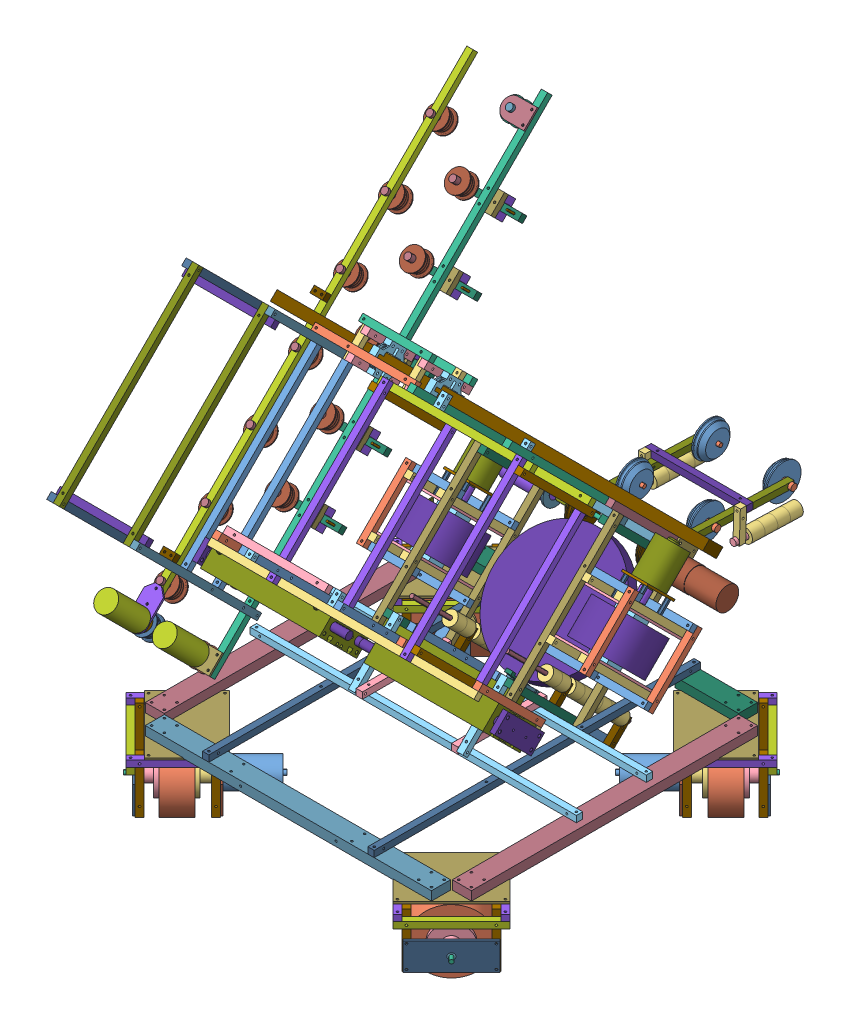
SolidWorks assembly R1, configuration ﾃﾞﾌｫﾙﾄ. Lengths in mm. (continued)
Components (placement in the parent): (continued)
- Copy of Assem3^R1-1: Copy of Assem3^R1 [ﾃﾞﾌｫﾙﾄ] at (-72.9957 96.2968 385.465) size (686.6 558.76 664.68) (virtual, flexible) (continued)
  - Assem5^Copy of Assem3_R1-1: Assem5^Copy of Assem3_R1 [ﾃﾞﾌｫﾙﾄ] at (161.552 -141.335 135.1971) x (1 0 0) z (0 0.000491 1) size (268.6 559.01 664.54) (virtual) (continued)
    - Copy of Copy of Copy of Copy (3) of Copy of Copy of Copy (2) of Copy of Copy (2) of 角材１^Assem5_Copy of Assem3_R1-5: Copy of Copy of Copy of Copy (3) of Copy of Copy of Copy (2) of Copy of Copy (2) of 角材１^Assem5_Copy of Assem3_R1 [ﾃﾞﾌｫﾙﾄ] at (-282.1724 380.5963 62.8061) x (-1 0 0) z (0 -0.707454 0.70676) size (90 10 10) (virtual)
    - Copy of Copy of Copy of Copy (3) of Copy of Copy of Copy (2) of Copy of Copy (2) of 角材１^Assem5_Copy of Assem3_R1-6: Copy of Copy of Copy of Copy (3) of Copy of Copy of Copy (2) of Copy of Copy (2) of 角材１^Assem5_Copy of Assem3_R1 [ﾃﾞﾌｫﾙﾄ] at (-282.1724 451.3417 -7.8698) x (-1 0 0) z (0 -0.707454 0.70676) size (90 10 10) (virtual)
    - Copy of Copy of Copy of Copy (3) of Copy of Copy of Copy (2) of Copy of Copy (2) of 角材１^Assem5_Copy of Assem3_R1-7: Copy of Copy of Copy of Copy (3) of Copy of Copy of Copy (2) of Copy of Copy (2) of 角材１^Assem5_Copy of Assem3_R1 [ﾃﾞﾌｫﾙﾄ] at (-282.1724 522.0871 -78.5458) x (-1 0 0) z (0 -0.707454 0.70676) size (90 10 10) (virtual)
    - Copy of Copy of Copy of Copy of Copy (2) of Copy of Part33^Assem5_Copy of Assem3_R1-2: Copy of Copy of Copy of Copy of Copy (2) of Copy of Part33^Assem5_Copy of Assem3_R1 [ﾃﾞﾌｫﾙﾄ] at (-379.2922 505.2902 839.4426) x (0 -0.70676 -0.707454) z (0.707107 0.500245 -0.499755) size (90 32 32) (virtual)
    - Copy of Copy of Copy of Copy (2) of Copy of Copy of Part5^Assem5_Copy of Assem3_R1-15: Copy of Copy of Copy of Copy (2) of Copy of Copy of Part5^Assem5_Copy of Assem3_R1 [ﾃﾞﾌｫﾙﾄ] at (-418.6839 580.481 -84.039) x (1 -0.000283 0.000282) z (-0.0004 -0.707454 0.70676) size (10 45 10) (virtual)
    - Copy of Copy of Copy of Copy of Copy (2) of Copy of Copy (2) of Part11^Assem5_Copy of Assem3_R1-15: Copy of Copy of Copy of Copy of Copy (2) of Copy of Copy (2) of Part11^Assem5_Copy of Assem3_R1 [ﾃﾞﾌｫﾙﾄ] at (-435.1724 568.3405 -96.2008) x (-0.731652 -0.482256 0.481783) z (-0.681679 0.51761 -0.517102) size (33.4 19.6 33.4) (virtual)
    - Copy of Copy of Copy of Copy (2) of Copy of Copy of Part5^Assem5_Copy of Assem3_R1-16: Copy of Copy of Copy of Copy (2) of Copy of Copy of Part5^Assem5_Copy of Assem3_R1 [ﾃﾞﾌｫﾙﾄ] at (-418.6839 226.7542 269.3408) x (1 -0.000283 0.000282) z (-0.0004 -0.707454 0.70676) size (10 45 10) (virtual)
    - Copy of Copy of Copy of Copy of Copy (2) of Copy of Copy (2) of Part11^Assem5_Copy of Assem3_R1-16: Copy of Copy of Copy of Copy of Copy (2) of Copy of Copy (2) of Part11^Assem5_Copy of Assem3_R1 [ﾃﾞﾌｫﾙﾄ] at (-435.1724 214.6137 257.1791) x (-0.731652 -0.482256 0.481783) z (-0.681679 0.51761 -0.517102) size (33.4 19.6 33.4) (virtual)
    - Copy of Part24^Assem5_Copy of Assem3_R1-1: Copy of Part24^Assem5_Copy of Assem3_R1 [ﾃﾞﾌｫﾙﾄ] at (-450.1724 147.54 338.6049) x (0 -0.707454 0.70676) z (0 0.70676 0.707454) size (61 30 3) (virtual)
    - Copy of Copy of Copy of Part36^Assem5_Copy of Assem3_R1-1: Copy of Copy of Copy of Part36^Assem5_Copy of Assem3_R1 [ﾃﾞﾌｫﾙﾄ] at (-386.0916 69.9556 399.151) x (-0.731652 -0.482256 0.481783) z (0 0.70676 0.707454) size (22 22 10) (virtual)
    - Copy (2) of Copy of Copy of Copy of Copy of Copy (2) of Copy of Copy (2) of Part11^Assem5_Copy of Assem3_R1-1: Copy (2) of Copy of Copy of Copy of Copy of Copy (2) of Copy of Copy (2) of Part11^Assem5_Copy of Assem3_R1 [ﾃﾞﾌｫﾙﾄ] at (-435.1724 108.4956 363.193) x (-0.731652 -0.482256 0.481783) z (-0.681679 0.51761 -0.517102) size (33.4 19.6 33.4) (virtual)
    - Copy of Copy of Copy of Part36^Assem5_Copy of Assem3_R1-2: Copy of Copy of Copy of Part36^Assem5_Copy of Assem3_R1 [ﾃﾞﾌｫﾙﾄ] at (-301.0916 62.888 392.0764) x (-0.731652 -0.482256 0.481783) z (0 0.70676 0.707454) size (22 22 10) (virtual)
    - Copy of Copy (2) of Copy of Copy of Copy of Copy of Copy (2) of Copy of Copy (2) of Part11^Assem5_Copy of Assem3_R1-1: Copy of Copy (2) of Copy of Copy of Copy of Copy of Copy (2) of Copy of Copy (2) of Part11^Assem5_Copy of Assem3_R1 [ﾃﾞﾌｫﾙﾄ] at (-350.1724 107.2235 361.9196) x (-0.731652 -0.482256 0.481783) z (-0.681679 0.51761 -0.517102) size (33.4 19.6 33.4) (virtual)
    - Copy of Copy of Copy of Copy of Copy (2) of Copy of Part33^Assem5_Copy of Assem3_R1-3: Copy of Copy of Copy of Copy of Copy (2) of Copy of Part33^Assem5_Copy of Assem3_R1 [ﾃﾞﾌｫﾙﾄ] at (-406.0526 498.2226 832.368) x (0 -0.70676 -0.707454) z (0.707107 -0.500245 0.499755) size (90 32 32) (virtual)
    - Copy of Copy of Part24^Assem5_Copy of Assem3_R1-1: Copy of Copy of Part24^Assem5_Copy of Assem3_R1 [ﾃﾞﾌｫﾙﾄ] at (-320.1724 119.2488 352.7331) x (-1 0 0) z (0 0.70676 0.707454) size (46 30 3) (virtual)
    - Copy of Copy of Copy of Part24^Assem5_Copy of Assem3_R1-1: Copy of Copy of Copy of Part24^Assem5_Copy of Assem3_R1 [ﾃﾞﾌｫﾙﾄ] at (-320.1724 614.4663 -141.9987) x (-1 0 0) z (0 0.70676 0.707454) size (45 30 3) (virtual)
    - Copy of Copy of Copy of Copy of Copy (2) of Copy of Copy of Part5^Assem5_Copy of Assem3_R1-1: Copy of Copy of Copy of Copy of Copy (2) of Copy of Copy of Part5^Assem5_Copy of Assem3_R1 [ﾃﾞﾌｫﾙﾄ] at (-333.7055 616.4547 -119.9775) x (0.998692 0.03617 -0.036135) z (0.051128 -0.706528 0.705835) size (10 38 10) (virtual)
    - Copy of Copy of Copy of Copy of Copy of Copy (2) of Copy of Copy (2) of Part11^Assem5_Copy of Assem3_R1-3: Copy of Copy of Copy of Copy of Copy of Copy (2) of Copy of Copy (2) of Part11^Assem5_Copy of Assem3_R1 [ﾃﾞﾌｫﾙﾄ] at (-350.1724 603.7132 -131.5388) x (-0.961431 -0.194584 0.194393) z (-0.275048 0.680168 -0.6795) size (33.4 19.6 33.4) (virtual)
  - Copy of Copy of MGPM20-150Z(0)_BODY^Copy of Assem3_R1-1: Copy of Copy of MGPM20-150Z(0)_BODY^Copy of Assem3_R1 [Default] at (271.3796 82.0315 468.7798) x (0 0.707107 -0.707107) z (1 0 0) size (36 83 187) (virtual)
  - Copy of Copy of MGPM20-150Z(0)_ROD^Copy of Assem3_R1-1: Copy of Copy of MGPM20-150Z(0)_ROD^Copy of Assem3_R1 [Default] at (271.3796 82.0315 468.7798) x (0 0.707107 -0.707107) z (1 0 0) size (30 81 227.5) (virtual)
  - Copy of Copy of Copy of Copy (3) of Copy of Copy (2) of 角材１^Copy of Assem3_R1-1: Copy of Copy of Copy of Copy (3) of Copy of Copy (2) of 角材１^Copy of Assem3_R1 [ﾃﾞﾌｫﾙﾄ] at (-290.6204 268.0006 261.5975) x (1 0 0) z (0 0.707107 0.707107) size (680 15 30) (virtual)
  - Copy of Copy of Copy of Copy (2) of Copy of Copy of Copy of Copy of 角材１^Copy of Assem3_R1-1: Copy of Copy of Copy of Copy (2) of Copy of Copy of Copy of Copy of 角材１^Copy of Assem3_R1 [ﾃﾞﾌｫﾙﾄ] at (-20.6204 -7.771 339.3792) x (0 0.707107 0.707107) z (0 -0.707107 0.707107) size (350 10 10) (virtual)
  - Copy of Copy of Copy of Copy (2) of Copy of Copy of Copy of Copy of 角材１^Copy of Assem3_R1-2: Copy of Copy of Copy of Copy (2) of Copy of Copy of Copy of Copy of 角材１^Copy of Assem3_R1 [ﾃﾞﾌｫﾙﾄ] at (129.3796 -7.771 339.3792) x (0 0.707107 0.707107) z (0 -0.707107 0.707107) size (350 10 10) (virtual)
  - Copy (3) of Part2^Copy of Assem3_R1-1: Copy (3) of Part2^Copy of Assem3_R1 [ﾃﾞﾌｫﾙﾄ] at (273.309 -803.9103 608.1734) (virtual)
  - Copy of Copy of Copy of Copy of Copy (2) of Copy of Copy (2) of 角材１^Copy of Assem3_R1-1: Copy of Copy of Copy of Copy of Copy (2) of Copy of Copy (2) of 角材１^Copy of Assem3_R1 [ﾃﾞﾌｫﾙﾄ] at (249.3796 45.262 406.5544) x (0 0.707107 0.707107) z (0 0.707107 -0.707107) size (140 10 10) (virtual)
  - Copy of Copy of Copy of Copy of Copy (2) of Copy of Copy (2) of 角材１^Copy of Assem3_R1-2: Copy of Copy of Copy of Copy of Copy (2) of Copy of Copy (2) of 角材１^Copy of Assem3_R1 [ﾃﾞﾌｫﾙﾄ] at (129.3796 45.262 406.5544) x (0 0.707107 0.707107) z (0 0.707107 -0.707107) size (140 10 10) (virtual)
  - Copy of Copy (2) of Copy of Copy (2) of Copy of Copy of Copy of Copy (2) of Copy of Copy (2) of 角材１^Copy of Assem3_R1-1: Copy of Copy (2) of Copy of Copy (2) of Copy of Copy of Copy of Copy (2) of Copy of Copy (2) of 角材１^Copy of Assem3_R1 [ﾃﾞﾌｫﾙﾄ] at (-160.6204 38.1909 413.6254) x (1 0 0) z (0 0.707107 0.707107) size (420 10 10) (virtual)
  - Copy of Copy (2) of Copy of Copy (2) of Copy of Copy of Copy of Copy (2) of Copy of Copy (2) of 角材１^Copy of Assem3_R1-2: Copy of Copy (2) of Copy of Copy (2) of Copy of Copy of Copy of Copy (2) of Copy of Copy (2) of 角材１^Copy of Assem3_R1 [ﾃﾞﾌｫﾙﾄ] at (-160.6204 130.1148 505.5493) x (1 0 0) z (0 0.707107 0.707107) size (420 10 10) (virtual)
  - Copy of Copy of Copy of Copy of Copy (2) of Copy of Copy (2) of 角材１^Copy of Assem3_R1-3: Copy of Copy of Copy of Copy of Copy (2) of Copy of Copy (2) of 角材１^Copy of Assem3_R1 [ﾃﾞﾌｫﾙﾄ] at (-160.6204 45.262 406.5544) x (0 0.707107 0.707107) z (0 0.707107 -0.707107) size (140 10 10) (virtual)
  - Copy of Copy of Copy of Copy of Copy (2) of Copy of Copy (2) of 角材１^Copy of Assem3_R1-4: Copy of Copy of Copy of Copy of Copy (2) of Copy of Copy (2) of 角材１^Copy of Assem3_R1 [ﾃﾞﾌｫﾙﾄ] at (-40.6204 45.262 406.5544) x (0 0.707107 0.707107) z (0 0.707107 -0.707107) size (140 10 10) (virtual)
  - Copy of Copy of MGPM20-150Z(0)_ROD^Copy of Assem3_R1-2: Copy of Copy of MGPM20-150Z(0)_ROD^Copy of Assem3_R1 [Default] at (-172.6204 82.0315 468.7798) x (0 0.707107 -0.707107) z (-1 0 0) size (30 81 227.5) (virtual)
  - Copy of Copy of MGPM20-150Z(0)_BODY^Copy of Assem3_R1-2: Copy of Copy of MGPM20-150Z(0)_BODY^Copy of Assem3_R1 [Default] at (-172.6204 82.0315 468.7798) x (0 0.707107 -0.707107) z (-1 0 0) size (36 83 187) (virtual)
  - Copy of Copy of Copy of Copy (2) of Copy of Copy (2) of 角材１^Copy of Assem3_R1-2: Copy of Copy of Copy of Copy (2) of Copy of Copy (2) of 角材１^Copy of Assem3_R1 [ﾃﾞﾌｫﾙﾄ] at (129.3796 270.6583 617.8085) x (-1 0 0) z (0 -0.707107 -0.707107) size (160 10 10) (virtual)
  - Copy of Copy of Copy of Copy of Copy of Copy of 角材１^Copy of Assem3_R1-9: Copy of Copy of Copy of Copy of Copy of Copy of 角材１^Copy of Assem3_R1 [ﾃﾞﾌｫﾙﾄ] at (-20.6204 232.6453 593.9377) x (0 0.707107 -0.707107) z (0 -0.707107 -0.707107) size (20 10 10) (virtual)
  - Copy of Copy of Copy of Copy of Copy of Copy of 角材１^Copy of Assem3_R1-10: Copy of Copy of Copy of Copy of Copy of Copy of 角材１^Copy of Assem3_R1 [ﾃﾞﾌｫﾙﾄ] at (109.3796 232.6453 593.9377) x (0 0.707107 -0.707107) z (0 -0.707107 -0.707107) size (20 10 10) (virtual)
  - Copy of Copy of Copy (4) of Copy of Copy of Copy of Copy (2) of Copy of Copy (2) of 角材１^Copy of Assem3_R1-1: Copy of Copy of Copy (4) of Copy of Copy of Copy of Copy (2) of Copy of Copy (2) of 角材１^Copy of Assem3_R1 [ﾃﾞﾌｫﾙﾄ] at (119.3796 84.1529 77.7497) x (0 0.707107 0.707107) z (1 0 0) size (345 10 10) (virtual)
  - Copy of Copy of Copy (4) of Copy of Copy of Copy of Copy (2) of Copy of Copy (2) of 角材１^Copy of Assem3_R1-2: Copy of Copy of Copy (4) of Copy of Copy of Copy of Copy (2) of Copy of Copy (2) of 角材１^Copy of Assem3_R1 [ﾃﾞﾌｫﾙﾄ] at (-30.6204 84.1529 77.7497) x (0 0.707107 0.707107) z (1 0 0) size (345 10 10) (virtual)
  - Copy of Copy of Copy (2) of Copy of Copy (2) of Copy of Copy of Copy of Copy (2) of Copy of Copy (2) of 角材１^Copy of Assem3_R1-2: Copy of Copy of Copy (2) of Copy of Copy (2) of Copy of Copy of Copy of Copy (2) of Copy of Copy (2) of 角材１^Copy of Assem3_R1 [ﾃﾞﾌｫﾙﾄ] at (-70.6204 306.8915 328.7726) x (1 0 0) z (0 0.707107 0.707107) size (240 10 10) (virtual)
  - Copy (5) of Copy of Copy of Copy (2) of Copy of Copy (2) of 角材１^Copy of Assem3_R1-1: Copy (5) of Copy of Copy of Copy (2) of Copy of Copy (2) of 角材１^Copy of Assem3_R1 [ﾃﾞﾌｫﾙﾄ] at (-50.6204 144.2569 519.6914) x (0 0.707107 -0.707107) z (-1 0 0) size (260 10 10) (virtual)
  - Copy of Copy (5) of Copy of Copy of Copy (2) of Copy of Copy (2) of 角材１^Copy of Assem3_R1-1: Copy of Copy (5) of Copy of Copy of Copy (2) of Copy of Copy (2) of 角材１^Copy of Assem3_R1 [ﾃﾞﾌｫﾙﾄ] at (-70.6204 38.1909 399.4833) x (0 0.707107 0.707107) z (0 0.707107 -0.707107) size (160 10 10) (virtual)
  - Copy (5) of Copy of Copy of Copy (2) of Copy of Copy (2) of 角材１^Copy of Assem3_R1-3: Copy (5) of Copy of Copy of Copy (2) of Copy of Copy (2) of 角材１^Copy of Assem3_R1 [ﾃﾞﾌｫﾙﾄ] at (-50.6204 38.1909 413.6254) x (0 0.707107 -0.707107) z (-1 0 0) size (260 10 10) (virtual)
  - Copy (5) of Copy of Copy of Copy (2) of Copy of Copy (2) of 角材１^Copy of Assem3_R1-4: Copy (5) of Copy of Copy of Copy (2) of Copy of Copy (2) of 角材１^Copy of Assem3_R1 [ﾃﾞﾌｫﾙﾄ] at (159.3796 144.2569 519.6914) x (0 0.707107 -0.707107) z (-1 0 0) size (260 10 10) (virtual)
  - Copy (5) of Copy of Copy of Copy (2) of Copy of Copy (2) of 角材１^Copy of Assem3_R1-5: Copy (5) of Copy of Copy of Copy (2) of Copy of Copy (2) of 角材１^Copy of Assem3_R1 [ﾃﾞﾌｫﾙﾄ] at (159.3796 38.1909 413.6254) x (0 0.707107 -0.707107) z (-1 0 0) size (260 10 10) (virtual)
  - Copy of Copy (5) of Copy of Copy of Copy (2) of Copy of Copy (2) of 角材１^Copy of Assem3_R1-2: Copy of Copy (5) of Copy of Copy of Copy (2) of Copy of Copy (2) of 角材１^Copy of Assem3_R1 [ﾃﾞﾌｫﾙﾄ] at (159.3796 38.1909 399.4833) x (0 0.707107 0.707107) z (0 0.707107 -0.707107) size (160 10 10) (virtual)
  - Copy of Copy of Copy (2) of Copy of Copy (2) of Copy of Copy of Copy of Copy (2) of Copy of Copy (2) of 角材１^Copy of Assem3_R1-3: Copy of Copy of Copy (2) of Copy of Copy (2) of Copy of Copy of Copy of Copy (2) of Copy of Copy (2) of 角材１^Copy of Assem3_R1 [ﾃﾞﾌｫﾙﾄ] at (-70.6204 214.9676 236.8487) x (1 0 0) z (0 0.707107 0.707107) size (240 10 10) (virtual)
  - Copy of Copy (5) of Copy of Copy of Copy (2) of Copy of Copy (2) of 角材１^Copy of Assem3_R1-3: Copy of Copy (5) of Copy of Copy of Copy (2) of Copy of Copy (2) of 角材１^Copy of Assem3_R1 [ﾃﾞﾌｫﾙﾄ] at (-70.6204 200.8255 236.8487) x (0 0.707107 0.707107) z (0 0.707107 -0.707107) size (160 10 10) (virtual)
  - Copy of Copy (5) of Copy of Copy of Copy (2) of Copy of Copy (2) of 角材１^Copy of Assem3_R1-4: Copy of Copy (5) of Copy of Copy of Copy (2) of Copy of Copy (2) of 角材１^Copy of Assem3_R1 [ﾃﾞﾌｫﾙﾄ] at (159.3796 200.8255 236.8487) x (0 0.707107 0.707107) z (0 0.707107 -0.707107) size (160 10 10) (virtual)
  - Copy of Copy of Copy of Copy of Copy of Copy of 角材１^Copy of Assem3_R1-11: Copy of Copy of Copy of Copy of Copy of Copy of 角材１^Copy of Assem3_R1 [ﾃﾞﾌｫﾙﾄ] at (109.3796 296.2849 275.7396) x (0 -0.707107 0.707107) z (0 0.707107 0.707107) size (20 10 10) (virtual)
  - Copy of Copy of Copy of Copy of Copy of Copy of 角材１^Copy of Assem3_R1-12: Copy of Copy of Copy of Copy of Copy of Copy of 角材１^Copy of Assem3_R1 [ﾃﾞﾌｫﾙﾄ] at (-20.6204 296.2849 275.7396) x (0 -0.707107 0.707107) z (0 0.707107 0.707107) size (20 10 10) (virtual)
- Copy of Copy of Copy of Copy (4) of Copy of Copy of Copy of Copy (2) of Copy of Copy (2) of 角材１^R1-1: Copy of Copy of Copy of Copy (4) of Copy of Copy of Copy of Copy (2) of Copy of Copy (2) of 角材１^R1 [ﾃﾞﾌｫﾙﾄ] at (-158.6161 31.0994 979.898) x (0 0 -1) z (0 -1 0) size (512.8 10 10) (virtual)
- Copy of Copy of Copy of Copy (4) of Copy of Copy of Copy of Copy (2) of Copy of Copy (2) of 角材１^R1-2: Copy of Copy of Copy of Copy (4) of Copy of Copy of Copy of Copy (2) of Copy of Copy (2) of 角材１^R1 [ﾃﾞﾌｫﾙﾄ] at (101.3839 31.0994 979.898) x (0 0 -1) z (0 -1 0) size (512.8 10 10) (virtual)
- D3V-016-1C23^R1-4: D3V-016-1C23^R1 [ﾃﾞﾌｫﾙﾄ] at (-28.4661 -2.0192 634.6527) x (-1 0 0) z (0 -0.707107 -0.707107) size (10.3 26.4 49.2) (virtual)
  - D3V_016_1C23_BASE^D3V-016-1C23_R1-1: D3V_016_1C23_BASE^D3V-016-1C23_R1 [ﾃﾞﾌｫﾙﾄ] at origin size (10.3 19.05 37.8) (virtual)
  - D3V_016_1C23_LEVER^D3V-016-1C23_R1-1: D3V_016_1C23_LEVER^D3V-016-1C23_R1 [ﾃﾞﾌｫﾙﾄ] at (-4.8 14.7 -11.8) x (0 0 -1) z (1 0 0) size (28.3 7.35 7.1) (virtual)
  - D3V_016_1C23_BUTTON^D3V-016-1C23_R1-1: D3V_016_1C23_BUTTON^D3V-016-1C23_R1 [ﾃﾞﾌｫﾙﾄ] at (-4.85 11.6 2) size (4.3 3.1 2.8) (virtual)
- Part8^R1-1: Part8^R1 [ﾃﾞﾌｫﾙﾄ] at (-8.4661 -3.1339 634.0253) x (0 0.707107 0.707107) z (-1 0 0) size (42.8 26.9 30.3) (virtual)
- Part9^R1-1: Part9^R1 [ﾃﾞﾌｫﾙﾄ] at (-18.4661 -0.0628 634.101) x (0 0.778227 0.627983) z (-1 0 0) size (50 10.5 10) (virtual)
- Part10^R1-1: Part10^R1 [ﾃﾞﾌｫﾙﾄ] at (-299.1739 21.0994 458.2016) x (-1 0 0) z (0 1 0) size (20 45 15) (virtual)
Mates (geometry in assembly coordinates):
- 距離1: distance = 20 mm anti-aligned: plane of Assem3-1/Copy of Copy of Copy of Copy (2) of Copy of Copy (2) of Copy of Copy (2) of 角材１^Assem3-2 through (-103.6161 41.0994 653.4838) normal (0 -1 0); plane of Runner-1/Copy of Part9^Runner-1 through (50.3133 21.0994 988.766) normal (0 1 0)
- 距離2: distance = 45 mm anti-aligned: plane of Assem3-1/Copy of Copy of Copy of Copy (2) of Copy of Copy (2) of Copy of Copy (2) of 角材１^Assem3-1 through (56.3839 41.0994 653.4838) normal (1 0 0); plane of 足回り-1/Copy (2) of Part9^足回り-2 through (101.3839 21.0994 497.0696) normal (-1 0 0)
- 一致2: coincident anti-aligned: plane of Copy of Shooter^R1-1/Copy of Copy (4) of Copy of Copy of Copy of Copy of Copy (2) of Copy of Copy (2) of 角材１^Shooter-1 through (-133.6161 95.5969 731.9152) normal (0 -0.707107 0.707107); plane of Copy of Assem3^R1-1/Copy of Copy of Copy of Copy (2) of Copy of Copy of Copy of Copy of 角材１^Copy of Assem3_R1-1 through (-93.6161 88.5258 724.8442) normal (0 0.707107 -0.707107)
- 同心円45: concentric aligned: cylinder of Copy of Shooter^R1-1/Copy of Copy (4) of Copy of Copy of Copy of Copy of Copy (2) of Copy of Copy (2) of 角材１^Shooter-1 through (51.3839 99.1324 721.3086) axis (0 0.707107 -0.707107) radius 1.6; cylinder of Copy of Assem3^R1-1/Copy of Copy of Copy of Copy (2) of Copy of Copy of Copy of Copy of 角材１^Copy of Assem3_R1-2 through (51.3839 92.0613 728.3797) axis (0 0.707107 -0.707107) radius 1.6
- 同心円46: concentric aligned: cylinder of Copy of Shooter^R1-1/Copy of Copy (4) of Copy of Copy of Copy of Copy of Copy (2) of Copy of Copy (2) of 角材１^Shooter-1 through (-98.6161 99.1324 721.3086) axis (0 0.707107 -0.707107) radius 1.6; cylinder of Copy of Assem3^R1-1/Copy of Copy of Copy of Copy (2) of Copy of Copy of Copy of Copy of 角材１^Copy of Assem3_R1-1 through (-98.6161 92.0613 728.3797) axis (0 0.707107 -0.707107) radius 1.6
- 一致3: coincident aligned: plane of Copy of Runner^R1-1/Copy of Part9^Runner-1 through (-248.6161 6.0994 979.898) normal (0 0 1); plane of Copy of Copy of Copy of Copy (4) of Copy of Copy of Copy of Copy (2) of Copy of Copy (2) of 角材１^R1-1 through (-148.6161 21.0994 979.898) normal (0 0 1)
- 一致4: coincident anti-aligned: plane of Copy of Runner^R1-1/Copy of Part9^Runner-1 through (50.3133 21.0994 988.766) normal (0 1 0); plane of Copy of Copy of Copy of Copy (4) of Copy of Copy of Copy of Copy (2) of Copy of Copy (2) of 角材１^R1-1 through (-158.6161 21.0994 979.898) normal (0 -1 0)
- 一致5: coincident aligned: plane of Copy of Runner^R1-1/Copy (2) of Part9^Runner-1 through (-148.6161 21.0994 467.0696) normal (1 0 0); plane of Copy of Copy of Copy of Copy (4) of Copy of Copy of Copy of Copy (2) of Copy of Copy (2) of 角材１^R1-1 through (-148.6161 21.0994 979.898) normal (1 0 0)
- 一致6: coincident aligned: plane of Copy of Runner^R1-1/Copy of Part9^Runner-1 through (-248.6161 6.0994 979.898) normal (0 0 1); plane of Copy of Copy of Copy of Copy (4) of Copy of Copy of Copy of Copy (2) of Copy of Copy (2) of 角材１^R1-2 through (111.3839 21.0994 979.898) normal (0 0 1)
- 一致7: coincident anti-aligned: plane of Copy of Runner^R1-1/Copy of Part9^Runner-1 through (50.3133 21.0994 988.766) normal (0 1 0); plane of Copy of Copy of Copy of Copy (4) of Copy of Copy of Copy of Copy (2) of Copy of Copy (2) of 角材１^R1-2 through (101.3839 21.0994 979.898) normal (0 -1 0)
- 一致8: coincident aligned: plane of Copy of Runner^R1-1/Copy (2) of Part9^Runner-2 through (101.3839 21.0994 497.0696) normal (-1 0 0); plane of Copy of Copy of Copy of Copy (4) of Copy of Copy of Copy of Copy (2) of Copy of Copy (2) of 角材１^R1-2 through (101.3839 21.0994 979.898) normal (-1 0 0)
- 距離3: distance = 165 mm aligned: plane of Copy of Shooter^R1-1/Copy of Copy (4) of Copy of Copy of Copy of Copy (2) of Copy of Copy (2) of 角材１^Shooter-2 through (232.7839 31.0994 663.4838) normal (0 0 -1); plane of Runner-1/Part9^Runner-3 through (-280.0303 21.0994 498.4838) normal (0 0 -1)
- 同心円47: concentric aligned: cylinder of D3V-016-1C23^R1-4/D3V_016_1C23_BASE^D3V-016-1C23_R1-1 through (-18.7661 -10.4338 611.6717) axis (-1 0 0) radius 1.55; cylinder of Part8^R1-1 through (-38.7661 -10.4338 611.6717) axis (-1 0 0) radius 1.75
- 同心円48: concentric aligned: cylinder of D3V-016-1C23^R1-4/D3V_016_1C23_BASE^D3V-016-1C23_R1-1 through (-18.7661 -2.0192 634.6527) axis (-1 0 0) radius 1.7; cylinder of Part8^R1-1 through (-38.7661 -2.0192 634.6527) axis (-1 0 0) radius 1.75
- 一致16: coincident anti-aligned: plane of D3V-016-1C23^R1-4/D3V_016_1C23_BASE^D3V-016-1C23_R1-1 through (-28.7661 -2.0192 635.2184) normal (-1 0 0); plane of Part8^R1-1 through (-28.7661 -21.6768 618.9549) normal (1 0 0)
- 同心円49: concentric aligned: cylinder of Copy of Shooter^R1-1/Copy (4) of Copy of Copy of Copy of Copy of Copy (2) of Copy of Copy (2) of 角材１^Shooter-2 through (-13.6161 14.2796 636.4558) axis (0 0.707107 -0.707107) radius 1.75; cylinder of Part8^R1-1 through (-13.6161 5.0518 645.6836) axis (0 0.707107 -0.707107) radius 1.75
- 同心円50: concentric aligned: cylinder of Copy of Shooter^R1-1/Copy (4) of Copy of Copy of Copy of Copy of Copy (2) of Copy of Copy (2) of 角材１^Shooter-2 through (-33.6161 14.2796 636.4558) axis (0 0.707107 -0.707107) radius 1.75; cylinder of Part8^R1-1 through (-33.6161 5.0518 645.6836) axis (0 0.707107 -0.707107) radius 1.75
- 一致17: coincident anti-aligned: plane of Copy of Shooter^R1-1/Copy (4) of Copy of Copy of Copy of Copy of Copy (2) of Copy of Copy (2) of 角材１^Shooter-2 through (-133.6161 17.8151 639.9914) normal (0 0.707107 -0.707107); plane of Part8^R1-1 through (-38.7661 10.7441 632.9203) normal (0 -0.707107 0.707107)
- 同心円51: concentric anti-aligned: cylinder of Part8^R1-1 through (-8.4661 -0.8878 605.2371) axis (-1 0 0) radius 1.75; cylinder of Part9^R1-1 through (-28.4661 -0.8878 605.2371) axis (1 0 0) radius 1.75
- 一致21: coincident anti-aligned: plane of Part8^R1-1 through (-18.4661 -21.6768 618.9549) normal (-1 0 0); plane of Part9^R1-1 through (-18.4661 -0.0628 634.101) normal (1 0 0)
